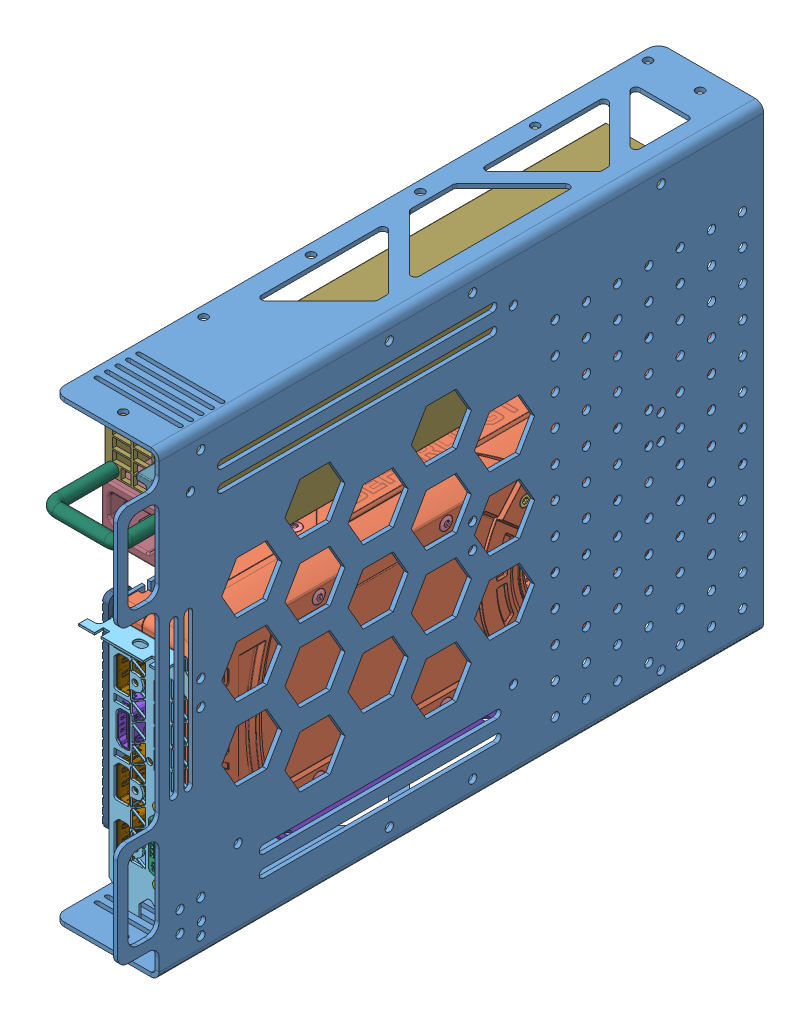
SolidWorks assembly kubebox_tray_gpu, configuration Default. Lengths in mm.
Overall size (58.48 220 311.35).
53 component instances, 25 part files, 2 mates.
Components (placement in the parent):
- GTX 980 assembly with backplate-1: GTX 980 assembly with backplate [Default] at (-38.5527 -30.3048 417.675) x (0 0 -1) z (0 -1 0) size (283.05 45.61 127.64)
  - titan pcb-1: titan pcb [Default] at origin size (267.04 35.65 111.3)
  - GTX 980 shroud-1: GTX 980 shroud [Default] at (0 1.651 0) size (270.72 38.11 99.71)
  - fan screw-1: fan screw [Default] at (159.7311 34.622 -32.369) x (1 0 0) z (0 -1 0) size (5.2 5.2 3.6)
  - fan screw-2: fan screw [Default] at (159.7311 34.622 -91.7335) x (1 0 0) z (0 -1 0) size (5.2 5.2 3.6)
  - fan screw-3: fan screw [Default] at (228.351 34.622 -32.369) x (1 0 0) z (0 -1 0) size (5.2 5.2 3.6)
  - fan screw-4: fan screw [Default] at (228.351 34.622 -91.7335) x (1 0 0) z (0 -1 0) size (5.2 5.2 3.6)
  - shroud screw-1: shroud screw [Default] at (73.2604 13.7824 -12.1993) x (0.923728 0.383049 0) z (0 0 -1) size (6 6 4.49)
  - shroud screw-2: shroud screw [Default] at (210.6175 13.7824 -12.1993) x (0.923728 0.383049 0) z (0 0 -1) size (6 6 4.49)
  - shroud screw-3: shroud screw [Default] at (62.0934 36.703 -24.1919) x (1 0 0) z (0 -1 0) size (6 6 4.49)
  - shroud screw-4: shroud screw [Default] at (123.1414 36.703 -24.1919) x (1 0 0) z (0 -1 0) size (6 6 4.49)
  - shroud screw-5: shroud screw [Default] at (62.0934 36.703 -99.9105) x (1 0 0) z (0 -1 0) size (6 6 4.49)
  - shroud screw-6: shroud screw [Default] at (73.2604 13.7824 -111.9032) size (6 6 4.49)
  - shroud screw-7: shroud screw [Default] at (210.6175 13.7824 -111.9032) size (6 6 4.49)
  - shroud screw-8: shroud screw [Default] at (123.1414 36.703 -99.9105) x (1 0 0) z (0 -1 0) size (6 6 4.49)
  - GTX 980 dual bracket-1: GTX 980 dual bracket [Default] at (-1 -1 15.2281) x (1 0 0) z (0 1 0) size (21.48 124.1 41.5)
  - dvi-2: dvi [Default] at (0 27.118 -24.8404) x (0 0 1) z (0 -1 0) size (36.83 11.58 9.91)
  - dvi screw-1: dvi screw [Default] at (-1 27.118 -41.0954) x (0 1 0) z (0 0 1) size (5.97 11.68 4.7)
  - dvi screw-3: dvi screw [Default] at (-1 27.118 -8.5854) x (0 1 0) z (0 0 1) size (5.97 11.68 4.7)
  - hdmi-1: hdmi [Default] at (-1 5.9592 -61.1544) x (0 0 1) z (-1 0 0) size (15 8.38 12.15)
  - displayport-1: displayport [Default] at (0.7 5.3484 -83.5652) x (0 0 1) z (-1 0 0) size (17.79 8.75 14.89)
  - GTX 980 backplate-1: GTX 980 backplate [Default] at (0 -5 0) size (267.05 5.85 98.06)
  - PCIE 6 pin-1: PCIE 6 pin [8] at (226.8669 6.451 -98.6023) x (1 0 0) z (0 1 0) size (13.8 12.7 11)
  - displayport-2: displayport [Default] at (0.7 5.3484 -38.0158) x (0 0 1) z (-1 0 0) size (17.79 8.75 14.89)
  - displayport-3: displayport [Default] at (0.7 5.3484 -14.6428) x (0 0 1) z (-1 0 0) size (17.79 8.75 14.89)
  - PCIE 6 pin-3: PCIE 6 pin [8] at (243.2612 6.451 -98.6023) x (1 0 0) z (0 1 0) size (13.8 12.7 11)
- PSK-2500G-1: PSK-2500G [Predeterminado] at (-39.0683 108.6191 420.973) x (0 -1 0) z (0 0 1) size (51.5 40.3 273)
  - psu_1u-micro-redundant-zippy.stp-1: psu_1u-micro-redundant-zippy.stp [Predeterminado] at origin size (122 41.72 328)
    - PSU_1U-MICRO-RED-1UNIT_ASM.stp-1: PSU_1U-MICRO-RED-1UNIT_ASM.stp [Predeterminado] at (-26.25 0 0) size (51.5 40.3 273)
      - PSU_1U-MICRO-RED-1UNIT_BODY.stp-1: PSU_1U-MICRO-RED-1UNIT_BODY.stp [Predeterminado] at origin size (51.5 40.3 240)
      - PSU_1U-MICOR_RED-1UNIT-PWRPORT.stp-1: PSU_1U-MICOR_RED-1UNIT-PWRPORT.stp [Predeterminado] at (11.9729 17.1645 0) size (25 32 23)
      - PSU_1U-MICRO-RED-1UNIT-CLICK.stp-1: PSU_1U-MICRO-RED-1UNIT-CLICK.stp [Predeterminado] at (-22 36.5 1.5) size (9.68 8.15 22)
      - PSU_1U-MICRO-RED-1UNIT_HANDLE.stp-1: PSU_1U-MICRO-RED-1UNIT_HANDLE.stp [Predeterminado] at (-3.7405 20.15 30) size (6 38.7 33)
      - PSU_1U-MICRO-RED_LED.stp-1: PSU_1U-MICRO-RED_LED.stp [Predeterminado] at (7 36 0.5) size (5 5 6.4)
    - PSU_1U-MICRO-RED-1UNIT_ASM.stp-2: PSU_1U-MICRO-RED-1UNIT_ASM.stp [Predeterminado] at (26.25 0 0) size (51.5 40.3 273) (hidden)
      - PSU_1U-MICRO-RED-1UNIT_BODY.stp-1: PSU_1U-MICRO-RED-1UNIT_BODY.stp [Predeterminado] at origin size (51.5 40.3 240)
      - PSU_1U-MICOR_RED-1UNIT-PWRPORT.stp-1: PSU_1U-MICOR_RED-1UNIT-PWRPORT.stp [Predeterminado] at (11.9729 17.1645 0) size (25 32 23)
      - PSU_1U-MICRO-RED-1UNIT-CLICK.stp-1: PSU_1U-MICRO-RED-1UNIT-CLICK.stp [Predeterminado] at (-22 36.5 1.5) size (9.68 8.15 22)
      - PSU_1U-MICRO-RED-1UNIT_HANDLE.stp-1: PSU_1U-MICRO-RED-1UNIT_HANDLE.stp [Predeterminado] at (-3.7405 20.15 30) size (6 38.7 33)
      - PSU_1U-MICRO-RED_LED.stp-1: PSU_1U-MICRO-RED_LED.stp [Predeterminado] at (7 36 0.5) size (5 5 6.4)
    - PSU_1U-MICRO-RED-MAINCASE.stp-1: PSU_1U-MICRO-RED-MAINCASE.stp [Predeterminado] at origin size (106 41.72 295) (hidden)
    - PSU_1U-MICRO-RED-SIDE-BRACKET.stp-1: PSU_1U-MICRO-RED-SIDE-BRACKET.stp [Predeterminado] at (53 0 0) size (8 41.3 12) (hidden)
    - PSU_1U-MICRO-RED-SIDE-BRACKET.stp-2: PSU_1U-MICRO-RED-SIDE-BRACKET.stp [Predeterminado] at (-53 41.3 0) x (-1 0 0) z (0 0 1) size (8 41.3 12) (hidden)
    - PSU_1U-MICRO-RED-SIDE-BRACKET-2.stp-1: PSU_1U-MICRO-RED-SIDE-BRACKET-2.stp [Predeterminado] at (-53 0 -14) size (7 10 267) (hidden)
    - PSU_1U-MICRO-RED-SIDE-BRACKET-2.stp-2: PSU_1U-MICRO-RED-SIDE-BRACKET-2.stp [Predeterminado] at (53 0 -281) x (-1 0 0) z (0 0 -1) size (7 10 267) (hidden)
    - PSU_1U-MICRO-RED-ALARMRESET.stp-1: PSU_1U-MICRO-RED-ALARMRESET.stp [Predeterminado] at (57.4 17.9 -1) size (6.6 12 8) (hidden)
- Riser_fin-1: Riser_fin [Default] at (-138.9377 -96.9695 329.69) x (0 0 -1) z (1 0 0) size (129.13 20.41 43.5)
  - Riser fin 2016.STEP-1: Riser fin 2016.STEP [Predeterminado] at (-47.4176 -7.3106 33.4441) size (129.13 20.41 43.5)
    - riser 2016.STEP-1: riser 2016.STEP [Predeterminado] at (79.7706 69.7258 73.4375) size (129.13 1 43.5)
    - usb_3.STEP-1: usb_3.STEP [Predeterminado] at (128.7305 74.0578 59.3899) x (0 0 -1) z (1 0 0) size (14.41 10.15 16.52) (hidden)
    - surface mount molex.STEP-1: surface mount molex.STEP [Predeterminado] at (131.5598 74.866 82.6621) x (0 0 -1) z (1 0 0) size (24.27 13.32 13.56) (hidden)
    - ASUS Maximus VII Impact - PCIe x16 Body_PCIe x16.STEP-1: ASUS Maximus VII Impact - PCIe x16 Body_PCIe x16.STEP [Predeterminado] at (104.614 70.7258 67.4543) x (0 0 1) z (-1 0 0) size (10.61 20.41 105.5)
- kubebox_tray-1: kubebox_tray [Predeterminado] at (2.6776 -45.5329 218.675) x (0 0 1) z (-1 0 0) size (310 220 45.5)
Mates (geometry in assembly coordinates):
- Coincident1: coincident aligned: plane of GTX 980 assembly with backplate-1/GTX 980 dual bracket-1 through (-0.7923 -45.5329 417.675) normal (0 -1 0); plane of kubebox_tray-1 through (2.6776 -45.5329 218.675) normal (0 -1 0)
- Coincident2: coincident anti-aligned: plane of GTX 980 assembly with backplate-1/GTX 980 dual bracket-1 through (-0.7923 -45.5329 418.675) normal (0 0 1); plane of kubebox_tray-1 through (-4.3224 64.4671 418.675) normal (0 0 -1)
